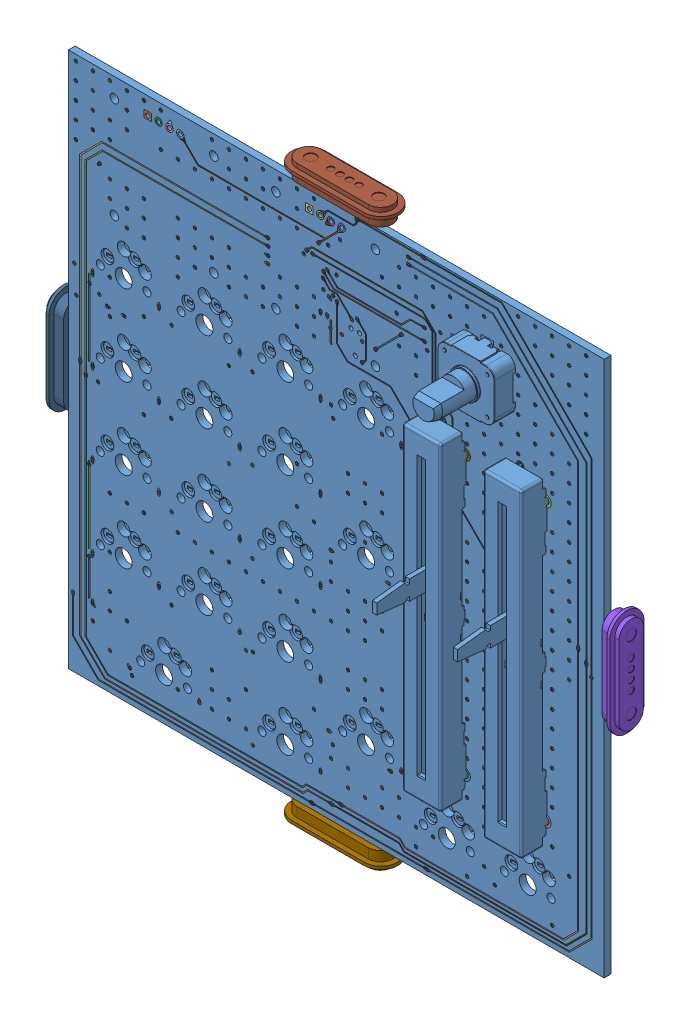
SolidWorks assembly Modulu1, configuration Default. Lengths in mm. (continued)
Components (placement in the parent): (continued)
- Numpad test 2.step-1: Numpad test 2.step [Default] at origin size (134.6 135 22.98) (continued)
  - Numpad test 21752.step-1: Numpad test 21752.step [Default] at origin size (1.31 0.29 0)
  - Numpad test 21753.step-1: Numpad test 21753.step [Default] at origin size (1.31 0.29 0)
  - Numpad test 21754.step-1: Numpad test 21754.step [Default] at origin size (0.82 0.18 0.01)
  - Numpad test 21755.step-1: Numpad test 21755.step [Default] at origin size (0.82 0.18 0.01)
  - Numpad test 21756.step-1: Numpad test 21756.step [Default] at origin size (1.76 0.36 0.01)
  - Numpad test 21757.step-1: Numpad test 21757.step [Default] at origin size (1.54 0.36 0.01)
  - Numpad test 21758.step-1: Numpad test 21758.step [Default] at origin size (0.38 0.64 0.01)
  - Numpad test 21759.step-1: Numpad test 21759.step [Default] at origin size (0.43 0.71 0.01)
  - Numpad test 21760.step-1: Numpad test 21760.step [Default] at origin size (2.14 1.77 0.01)
  - Numpad test 21761.step-1: Numpad test 21761.step [Default] at origin size (0.34 1.47 0.01)
  - Numpad test 21762.step-1: Numpad test 21762.step [Default] at origin size (0.34 1.47 0.01)
  - Numpad test 21763.step-1: Numpad test 21763.step [Default] at origin size (0.34 0.89 0.01)
  - Numpad test 21764.step-1: Numpad test 21764.step [Default] at origin size (0.34 0.89 0.01)
  - Numpad test 21765.step-1: Numpad test 21765.step [Default] at origin size (2.39 1.29 0.01)
  - Numpad test 21766.step-1: Numpad test 21766.step [Default] at origin size (2.33 1.32 0.01)
  - Numpad test 21767.step-1: Numpad test 21767.step [Default] at origin size (2.33 1.32 0.01)
  - Numpad test 21768.step-1: Numpad test 21768.step [Default] at origin size (2.33 1.32 0.01)
  - Numpad test 21769.step-1: Numpad test 21769.step [Default] at origin size (2.32 1.29 0.01)
  - Numpad test 21770.step-1: Numpad test 21770.step [Default] at origin size (2.3 1.29 0.01)
  - Numpad test 21771.step-1: Numpad test 21771.step [Default] at origin size (1.38 0.36 0.01)
  - Numpad test 21772.step-1: Numpad test 21772.step [Default] at origin size (0.36 0.71 0.01)
  - Numpad test 21773.step-1: Numpad test 21773.step [Default] at origin size (1.65 0.8 0.01)
  - Numpad test 21774.step-1: Numpad test 21774.step [Default] at origin size (2.15 1.25 0.02)
  - Numpad test 21775.step-1: Numpad test 21775.step [Default] at origin size (2.15 1.25 0.02)
  - Numpad test 21776.step-1: Numpad test 21776.step [Default] at origin size (2.15 1.25 0.02)
  - Numpad test 21777.step-1: Numpad test 21777.step [Default] at origin size (2.15 1.25 0.02)
  - Numpad test 21778.step-1: Numpad test 21778.step [Default] at origin size (2.15 1.25 0.02)
  - Numpad test 21779.step-1: Numpad test 21779.step [Default] at origin size (2.15 1.25 0.02)
  - Numpad test 21780.step-1: Numpad test 21780.step [Default] at origin size (2.15 1.25 0.02)
  - Numpad test 21781.step-1: Numpad test 21781.step [Default] at origin size (1.32 2.07 0.01)
  - Numpad test 21782.step-1: Numpad test 21782.step [Default] at origin size (1.19 0.27 0.01)
  - Numpad test 21783.step-1: Numpad test 21783.step [Default] at origin size (0.37 0.42 0.01)
  - Numpad test 21784.step-1: Numpad test 21784.step [Default] at origin size (1.26 0.4 0.01)
  - Numpad test 21785.step-1: Numpad test 21785.step [Default] at origin size (0.39 0.32 0.01)
  - Numpad test 21786.step-1: Numpad test 21786.step [Default] at origin size (0.09 0.09 0.01)
  - Numpad test 21787.step-1: Numpad test 21787.step [Default] at origin size (0.72 1.4 0)
  - Numpad test 21788.step-1: Numpad test 21788.step [Default] at origin size (0.72 1.42 0)
  - Numpad test 21789.step-1: Numpad test 21789.step [Default] at origin size (0.72 1.56 0)
  - Numpad test 21790.step-1: Numpad test 21790.step [Default] at origin size (0.72 1.56 0)
  - Numpad test 21791.step-1: Numpad test 21791.step [Default] at origin size (0.72 1.56 0)
  - Numpad test 21792.step-1: Numpad test 21792.step [Default] at origin size (0.72 1.56 0)
  - Numpad test 21793.step-1: Numpad test 21793.step [Default] at origin size (1.1 0.34 0.01)
  - Numpad test 21794.step-1: Numpad test 21794.step [Default] at origin size (0.36 0.33 0.01)
  - Numpad test 21795.step-1: Numpad test 21795.step [Default] at origin size (1.34 0.34 0.01)
  - Numpad test 21796.step-1: Numpad test 21796.step [Default] at origin size (0.2 0.37 0.01)
  - Numpad test 21797.step-1: Numpad test 21797.step [Default] at origin size (1.61 1.52 0.01)
  - Numpad test 21798.step-1: Numpad test 21798.step [Default] at origin size (1.38 1.39 0.01)
  - Numpad test 21799.step-1: Numpad test 21799.step [Default] at origin size (1.39 1.38 0.01)
  - Numpad test 21800.step-1: Numpad test 21800.step [Default] at origin size (1.28 0.37 0.01)
  - Numpad test 21801.step-1: Numpad test 21801.step [Default] at origin size (0.76 0.14 0.01)
  - Numpad test 21802.step-1: Numpad test 21802.step [Default] at origin size (0.32 0.77 0.01)
  - Numpad test 21803.step-1: Numpad test 21803.step [Default] at origin size (0.32 0.56 0.01)
  - Numpad test 21804.step-1: Numpad test 21804.step [Default] at origin size (1.45 1.59 0.01)
  - Numpad test 21805.step-1: Numpad test 21805.step [Default] at origin size (1.86 0.83 0.01)
  - Numpad test 21806.step-1: Numpad test 21806.step [Default] at origin size (0.61 1.43 0)
  - Numpad test 21807.step-1: Numpad test 21807.step [Default] at origin size (0.55 1.09 0)
  - Numpad test 21808.step-1: Numpad test 21808.step [Default] at origin size (0.8 1.02 0)
  - Numpad test 21809.step-1: Numpad test 21809.step [Default] at origin size (1.23 1.11 0)
  - Numpad test 21810.step-1: Numpad test 21810.step [Default] at origin size (1.69 0.83 0.01)
  - Numpad test 21811.step-1: Numpad test 21811.step [Default] at origin size (1.4 0.29 0.01)
  - Numpad test 21812.step-1: Numpad test 21812.step [Default] at origin size (1.4 0.29 0.01)
  - Numpad test 21813.step-1: Numpad test 21813.step [Default] at origin size (0.29 1.4 0.01)
  - Numpad test 21814.step-1: Numpad test 21814.step [Default] at origin size (0.29 1.4 0.01)
  - Numpad test 21815.step-1: Numpad test 21815.step [Default] at origin size (0.29 1.4 0.01)
  - Numpad test 21816.step-1: Numpad test 21816.step [Default] at origin size (0.29 1.4 0.01)
  - Numpad test 21817.step-1: Numpad test 21817.step [Default] at origin size (1.4 0.29 0.01)
  - Numpad test 21818.step-1: Numpad test 21818.step [Default] at origin size (1.4 0.29 0.01)
  - Numpad test 21819.step-1: Numpad test 21819.step [Default] at origin size (1.3 1.35 0.01)
  - Numpad test 21820.step-1: Numpad test 21820.step [Default] at origin size (1.51 1.08 0.01)
  - Numpad test 21821.step-1: Numpad test 21821.step [Default] at origin size (0.93 1.59 0.01)
  - Numpad test 21822.step-1: Numpad test 21822.step [Default] at origin size (0.78 0.71 0.01)
  - Numpad test 21823.step-1: Numpad test 21823.step [Default] at origin size (0.31 0.76 0.01)
  - Numpad test 21824.step-1: Numpad test 21824.step [Default] at origin size (0.83 0.29 0.01)
  - Numpad test 21825.step-1: Numpad test 21825.step [Default] at origin size (0.93 1.51 0.01)
  - Numpad test 21826.step-1: Numpad test 21826.step [Default] at origin size (0.66 0.37 0.01)
  - Numpad test 21827.step-1: Numpad test 21827.step [Default] at origin size (0.61 0.84 0.01)
  - Numpad test 21828.step-1: Numpad test 21828.step [Default] at origin size (0.83 0.72 0.01)
  - Numpad test 21829.step-1: Numpad test 21829.step [Default] at origin size (1.36 0.32 0)
  - Numpad test 21830.step-1: Numpad test 21830.step [Default] at origin size (1.36 0.32 0)
  - Numpad test 21831.step-1: Numpad test 21831.step [Default] at origin size (0.79 1.51 0.01)
  - Numpad test 21832.step-1: Numpad test 21832.step [Default] at origin size (0.93 1.41 0.01)
  - Numpad test 21833.step-1: Numpad test 21833.step [Default] at origin size (1.4 0.88 0.01)
  - Numpad test 21834.step-1: Numpad test 21834.step [Default] at origin size (1.17 0.32 0.01)
  - Numpad test 21835.step-1: Numpad test 21835.step [Default] at origin size (1.17 0.32 0.01)
  - Numpad test 21836.step-1: Numpad test 21836.step [Default] at origin size (1.4 0.88 0.01)
  - Numpad test 21837.step-1: Numpad test 21837.step [Default] at origin size (1.4 0.88 0.01)
  - Numpad test 21838.step-1: Numpad test 21838.step [Default] at origin size (1.4 0.88 0.01)
  - Numpad test 21839.step-1: Numpad test 21839.step [Default] at origin size (1.4 0.88 0.01)
  - Numpad test 21840.step-1: Numpad test 21840.step [Default] at origin size (1.4 0.88 0.01)
  - Numpad test 21841.step-1: Numpad test 21841.step [Default] at origin size (1.4 0.88 0.01)
  - Numpad test 21842.step-1: Numpad test 21842.step [Default] at origin size (1.17 0.32 0.01)
  - Numpad test 21843.step-1: Numpad test 21843.step [Default] at origin size (1.17 0.32 0.01)
  - Numpad test 21844.step-1: Numpad test 21844.step [Default] at origin size (1.4 0.88 0.01)
  - Numpad test 21845.step-1: Numpad test 21845.step [Default] at origin size (1.4 0.88 0.01)
  - Numpad test 21846.step-1: Numpad test 21846.step [Default] at origin size (1.4 0.88 0.01)
  - Numpad test 21847.step-1: Numpad test 21847.step [Default] at origin size (1.4 0.88 0.01)
  - Numpad test 21848.step-1: Numpad test 21848.step [Default] at origin size (1.4 0.88 0.01)
  - Numpad test 21849.step-1: Numpad test 21849.step [Default] at origin size (1.4 0.88 0.01)
  - Numpad test 21850.step-1: Numpad test 21850.step [Default] at origin size (1.4 0.88 0.01)
  - Numpad test 21851.step-1: Numpad test 21851.step [Default] at origin size (1.4 0.88 0.01)
  - Numpad test 21852.step-1: Numpad test 21852.step [Default] at origin size (1.4 0.88 0.01)
  - Numpad test 21853.step-1: Numpad test 21853.step [Default] at origin size (1.4 0.88 0.01)
  - Numpad test 21854.step-1: Numpad test 21854.step [Default] at origin size (1.4 0.88 0.01)
  - Numpad test 21855.step-1: Numpad test 21855.step [Default] at origin size (1.4 0.88 0.01)
  - Numpad test 21856.step-1: Numpad test 21856.step [Default] at origin size (1.4 0.88 0.01)
  - Numpad test 21857.step-1: Numpad test 21857.step [Default] at origin size (1.17 0.32 0.01)
  - Numpad test 21858.step-1: Numpad test 21858.step [Default] at origin size (1.17 0.32 0.01)
  - Numpad test 21859.step-1: Numpad test 21859.step [Default] at origin size (1.4 0.88 0.01)
  - Numpad test 21860.step-1: Numpad test 21860.step [Default] at origin size (1.17 0.32 0.01)
  - Numpad test 21861.step-1: Numpad test 21861.step [Default] at origin size (1.17 0.32 0.01)
  - Numpad test 21862.step-1: Numpad test 21862.step [Default] at origin size (1.4 0.88 0.01)
  - Numpad test 21863.step-1: Numpad test 21863.step [Default] at origin size (1.4 0.88 0.01)
  - Numpad test 21864.step-1: Numpad test 21864.step [Default] at origin size (1.4 0.88 0.01)
  - Numpad test 21865.step-1: Numpad test 21865.step [Default] at origin size (1.4 0.88 0.01)
  - Numpad test 21866.step-1: Numpad test 21866.step [Default] at origin size (1.4 0.88 0.01)
  - Numpad test 21867.step-1: Numpad test 21867.step [Default] at origin size (1.17 0.32 0.01)
  - Numpad test 21868.step-1: Numpad test 21868.step [Default] at origin size (1.17 0.32 0.01)
  - Numpad test 21869.step-1: Numpad test 21869.step [Default] at origin size (1.4 0.88 0.01)
  - Numpad test 21870.step-1: Numpad test 21870.step [Default] at origin size (1.4 0.88 0.01)
  - Numpad test 21871.step-1: Numpad test 21871.step [Default] at origin size (1.4 0.88 0.01)
  - Numpad test 21872.step-1: Numpad test 21872.step [Default] at origin size (1.4 0.88 0.01)
  - Numpad test 21873.step-1: Numpad test 21873.step [Default] at origin size (0.93 1.29 0.01)
  - Numpad test 21874.step-1: Numpad test 21874.step [Default] at origin size (0.93 1.29 0.01)
  - Numpad test 21875.step-1: Numpad test 21875.step [Default] at origin size (0.93 1.29 0.01)
  - Numpad test 21876.step-1: Numpad test 21876.step [Default] at origin size (0.93 1.29 0.01)
  - Numpad test 21877.step-1: Numpad test 21877.step [Default] at origin size (0.93 1.29 0.01)
  - Numpad test 21878.step-1: Numpad test 21878.step [Default] at origin size (0.93 1.29 0.01)
  - Numpad test 21879.step-1: Numpad test 21879.step [Default] at origin size (0.34 1.2 0)
  - Numpad test 21880.step-1: Numpad test 21880.step [Default] at origin size (0.34 1.2 0)
  - Numpad test 21881.step-1: Numpad test 21881.step [Default] at origin size (0.93 1.29 0.01)
  - Numpad test 21882.step-1: Numpad test 21882.step [Default] at origin size (0.93 1.21 0.01)
  - Numpad test 21883.step-1: Numpad test 21883.step [Default] at origin size (0.93 1.21 0.01)
  - Numpad test 21884.step-1: Numpad test 21884.step [Default] at origin size (0.93 1.21 0.01)
  - Numpad test 21885.step-1: Numpad test 21885.step [Default] at origin size (0.93 1.21 0.01)
  - Numpad test 21886.step-1: Numpad test 21886.step [Default] at origin size (0.93 1.19 0.01)
  - Numpad test 21887.step-1: Numpad test 21887.step [Default] at origin size (0.34 1.1 0)
  - Numpad test 21888.step-1: Numpad test 21888.step [Default] at origin size (0.34 1.1 0)
  - Numpad test 21889.step-1: Numpad test 21889.step [Default] at origin size (1.17 0.84 0.02)
  - Numpad test 21890.step-1: Numpad test 21890.step [Default] at origin size (0.72 0.18 0.01)
  - Numpad test 21891.step-1: Numpad test 21891.step [Default] at origin size (0.88 0.24 0.01)
  - Numpad test 21892.step-1: Numpad test 21892.step [Default] at origin size (1.18 0.59 0.01)
  - Numpad test 21893.step-1: Numpad test 21893.step [Default] at origin size (1.18 0.59 0.01)
  - Numpad test 21894.step-1: Numpad test 21894.step [Default] at origin size (1.18 0.59 0.01)
  - Numpad test 21895.step-1: Numpad test 21895.step [Default] at origin size (1.18 0.59 0.01)
  - Numpad test 21896.step-1: Numpad test 21896.step [Default] at origin size (1.18 0.59 0.01)
  - Numpad test 21897.step-1: Numpad test 21897.step [Default] at origin size (1.18 0.59 0.01)
  - Numpad test 21898.step-1: Numpad test 21898.step [Default] at origin size (0.88 0.24 0.01)
  - Numpad test 21899.step-1: Numpad test 21899.step [Default] at origin size (0.72 0.18 0.01)
  - Numpad test 21900.step-1: Numpad test 21900.step [Default] at origin size (0.61 1.11 0.01)
  - Numpad test 21901.step-1: Numpad test 21901.step [Default] at origin size (0.18 0.82 0.01)
  - Numpad test 21902.step-1: Numpad test 21902.step [Default] at origin size (0.18 0.82 0.01)
  - Numpad test 21903.step-1: Numpad test 21903.step [Default] at origin size (1.11 0.61 0.01)
  - Numpad test 21904.step-1: Numpad test 21904.step [Default] at origin size (0.18 0.82 0.01)
  - Numpad test 21905.step-1: Numpad test 21905.step [Default] at origin size (0.18 0.82 0.01)
  - Numpad test 21906.step-1: Numpad test 21906.step [Default] at origin size (0.18 0.82 0.01)
  - Numpad test 21907.step-1: Numpad test 21907.step [Default] at origin size (0.18 0.82 0.01)
  - Numpad test 21908.step-1: Numpad test 21908.step [Default] at origin size (1.11 0.61 0.01)
  - Numpad test 21909.step-1: Numpad test 21909.step [Default] at origin size (0.61 1.11 0.01)
  - Numpad test 21910.step-1: Numpad test 21910.step [Default] at origin size (0.18 0.82 0.01)
  - Numpad test 21911.step-1: Numpad test 21911.step [Default] at origin size (0.18 0.82 0.01)
  - Numpad test 21912.step-1: Numpad test 21912.step [Default] at origin size (1.11 0.61 0.01)
  - Numpad test 21913.step-1: Numpad test 21913.step [Default] at origin size (1.11 0.61 0.01)
  - Numpad test 21914.step-1: Numpad test 21914.step [Default] at origin size (1.11 0.61 0.01)
  - Numpad test 21915.step-1: Numpad test 21915.step [Default] at origin size (0.11 0.12 0.01)
  - Numpad test 21916.step-1: Numpad test 21916.step [Default] at origin size (0.11 0.56 0.01)
  - Numpad test 21917.step-1: Numpad test 21917.step [Default] at origin size (0.18 0.68 0.01)
  - Numpad test 21918.step-1: Numpad test 21918.step [Default] at origin size (0.63 0.34 0.01)
  - Numpad test 21919.step-1: Numpad test 21919.step [Default] at origin size (0.79 0.39 0.01)
  - Numpad test 21920.step-1: Numpad test 21920.step [Default] at origin size (0.63 0.34 0.01)
  - Numpad test 21921.step-1: Numpad test 21921.step [Default] at origin size (0.79 0.39 0.01)
  - Numpad test 21922.step-1: Numpad test 21922.step [Default] at origin size (0.91 0.84 0.01)
  - Numpad test 21923.step-1: Numpad test 21923.step [Default] at origin size (0.32 0.77 0.01)
  - Numpad test 21924.step-1: Numpad test 21924.step [Default] at origin size (0.32 0.77 0.01)
  - Numpad test 21925.step-1: Numpad test 21925.step [Default] at origin size (0.63 0.69 0.01)
  - Numpad test 21926.step-1: Numpad test 21926.step [Default] at origin size (0.57 0.5 0.01)
  - Numpad test 21927.step-1: Numpad test 21927.step [Default] at origin size (0.86 0.86 0.01)
  - Numpad test 21928.step-1: Numpad test 21928.step [Default] at origin size (0.86 0.86 0.01)
  - Numpad test 21929.step-1: Numpad test 21929.step [Default] at origin size (0.5 0.67 0)
  - Numpad test 21930.step-1: Numpad test 21930.step [Default] at origin size (0.67 0.5 0)
  - Numpad test 21931.step-1: Numpad test 21931.step [Default] at origin size (0.67 0.5 0)
  - Numpad test 21932.step-1: Numpad test 21932.step [Default] at origin size (0.5 0.67 0)
  - Numpad test 21933.step-1: Numpad test 21933.step [Default] at origin size (0.5 0.67 0)
  - Numpad test 21934.step-1: Numpad test 21934.step [Default] at origin size (0.67 0.5 0)
  - Numpad test 21935.step-1: Numpad test 21935.step [Default] at origin size (0.5 0.67 0)
  - Numpad test 21936.step-1: Numpad test 21936.step [Default] at origin size (0.67 0.5 0)
  - Numpad test 21937.step-1: Numpad test 21937.step [Default] at origin size (0.5 0.67 0)
  - Numpad test 21938.step-1: Numpad test 21938.step [Default] at origin size (0.67 0.5 0)
  - Numpad test 21939.step-1: Numpad test 21939.step [Default] at origin size (0.67 0.5 0)
  - Numpad test 21940.step-1: Numpad test 21940.step [Default] at origin size (0.5 0.67 0)
  - Numpad test 21941.step-1: Numpad test 21941.step [Default] at origin size (0.86 0.86 0.01)
  - Numpad test 21942.step-1: Numpad test 21942.step [Default] at origin size (0.86 0.86 0.01)
  - Numpad test 21943.step-1: Numpad test 21943.step [Default] at origin size (0.53 0.65 0.01)
  - Numpad test 21944.step-1: Numpad test 21944.step [Default] at origin size (0.69 0.47 0)
  - Numpad test 21945.step-1: Numpad test 21945.step [Default] at origin size (0.31 0.76 0.01)
  - Numpad test 21946.step-1: Numpad test 21946.step [Default] at origin size (0.31 0.76 0.01)
  - Numpad test 21947.step-1: Numpad test 21947.step [Default] at origin size (0.76 0.31 0.01)
  - Numpad test 21948.step-1: Numpad test 21948.step [Default] at origin size (0.76 0.31 0.01)
  - Numpad test 21949.step-1: Numpad test 21949.step [Default] at origin size (0.86 0.85 0.01)
  - Numpad test 21950.step-1: Numpad test 21950.step [Default] at origin size (0.75 0.31 0.01)
  - Numpad test 21951.step-1: Numpad test 21951.step [Default] at origin size (0.75 0.31 0.01)
  - Numpad test 21952.step-1: Numpad test 21952.step [Default] at origin size (0.85 0.86 0.01)
  - Numpad test 21953.step-1: Numpad test 21953.step [Default] at origin size (0.51 0.69 0.01)
  - Numpad test 21954.step-1: Numpad test 21954.step [Default] at origin size (0.03 0.21 0.01)
  - Numpad test 21955.step-1: Numpad test 21955.step [Default] at origin size (0.37 0.44 0.01)
  - Numpad test 21956.step-1: Numpad test 21956.step [Default] at origin size (0.57 0.67 0.01)
  - Numpad test 21957.step-1: Numpad test 21957.step [Default] at origin size (0.63 0.57 0.01)
  - Numpad test 21958.step-1: Numpad test 21958.step [Default] at origin size (0.8 0.27 0.01)
  - Numpad test 21959.step-1: Numpad test 21959.step [Default] at origin size (0.8 0.27 0.01)
  - Numpad test 21960.step-1: Numpad test 21960.step [Default] at origin size (0.8 0.27 0.01)
  - Numpad test 21961.step-1: Numpad test 21961.step [Default] at origin size (0.8 0.27 0.01)
  - Numpad test 21962.step-1: Numpad test 21962.step [Default] at origin size (0.85 0.78 0.01)
  - Numpad test 21963.step-1: Numpad test 21963.step [Default] at origin size (0.8 0.27 0.01)
  - Numpad test 21964.step-1: Numpad test 21964.step [Default] at origin size (0.8 0.27 0.01)
  - Numpad test 21965.step-1: Numpad test 21965.step [Default] at origin size (0.83 0.79 0.01)
  - Numpad test 21966.step-1: Numpad test 21966.step [Default] at origin size (0.79 0.81 0.01)
  - Numpad test 21967.step-1: Numpad test 21967.step [Default] at origin size (0.79 0.81 0.01)
  - Numpad test 21968.step-1: Numpad test 21968.step [Default] at origin size (0.77 0.29 0)
  - Numpad test 21969.step-1: Numpad test 21969.step [Default] at origin size (0.77 0.29 0)
  - Numpad test 21970.step-1: Numpad test 21970.step [Default] at origin size (0.78 0.79 0.01)
  - Numpad test 21971.step-1: Numpad test 21971.step [Default] at origin size (0.78 0.79 0.01)
  - Numpad test 21972.step-1: Numpad test 21972.step [Default] at origin size (0.78 0.79 0.01)
  - Numpad test 21973.step-1: Numpad test 21973.step [Default] at origin size (0.77 0.29 0)
  - Numpad test 21974.step-1: Numpad test 21974.step [Default] at origin size (0.77 0.29 0)
  - Numpad test 21975.step-1: Numpad test 21975.step [Default] at origin size (0.78 0.79 0.01)
  - Numpad test 21976.step-1: Numpad test 21976.step [Default] at origin size (0.78 0.79 0.01)
  - Numpad test 21977.step-1: Numpad test 21977.step [Default] at origin size (0.78 0.79 0.01)
  - Numpad test 21978.step-1: Numpad test 21978.step [Default] at origin size (0.78 0.79 0.01)
  - Numpad test 21979.step-1: Numpad test 21979.step [Default] at origin size (0.78 0.79 0.01)
  - Numpad test 21980.step-1: Numpad test 21980.step [Default] at origin size (0.78 0.79 0.01)
  - Numpad test 21981.step-1: Numpad test 21981.step [Default] at origin size (0.78 0.79 0.01)
  - Numpad test 21982.step-1: Numpad test 21982.step [Default] at origin size (0.77 0.29 0)
  - Numpad test 21983.step-1: Numpad test 21983.step [Default] at origin size (0.77 0.29 0)
  - Numpad test 21984.step-1: Numpad test 21984.step [Default] at origin size (0.77 0.29 0)
  - Numpad test 21985.step-1: Numpad test 21985.step [Default] at origin size (0.77 0.29 0)
  - Numpad test 21986.step-1: Numpad test 21986.step [Default] at origin size (0.78 0.79 0.01)
  - Numpad test 21987.step-1: Numpad test 21987.step [Default] at origin size (0.73 0.29 0)
  - Numpad test 21988.step-1: Numpad test 21988.step [Default] at origin size (0.77 0.29 0)
  - Numpad test 21989.step-1: Numpad test 21989.step [Default] at origin size (0.77 0.29 0)
  - Numpad test 21990.step-1: Numpad test 21990.step [Default] at origin size (0.77 0.29 0)
  - Numpad test 21991.step-1: Numpad test 21991.step [Default] at origin size (0.78 0.79 0.01)
  - Numpad test 21992.step-1: Numpad test 21992.step [Default] at origin size (0.78 0.79 0.01)
  - Numpad test 21993.step-1: Numpad test 21993.step [Default] at origin size (0.77 0.29 0)
  - Numpad test 21994.step-1: Numpad test 21994.step [Default] at origin size (0.77 0.29 0)
  - Numpad test 21995.step-1: Numpad test 21995.step [Default] at origin size (0.78 0.79 0.01)
  - Numpad test 21996.step-1: Numpad test 21996.step [Default] at origin size (0.78 0.79 0.01)
  - Numpad test 21997.step-1: Numpad test 21997.step [Default] at origin size (0.28 0.77 0)
  - Numpad test 21998.step-1: Numpad test 21998.step [Default] at origin size (0.28 0.77 0)
  - Numpad test 21999.step-1: Numpad test 21999.step [Default] at origin size (0.28 0.77 0)
  - Numpad test 22000.step-1: Numpad test 22000.step [Default] at origin size (0.28 0.77 0)
  - Numpad test 22001.step-1: Numpad test 22001.step [Default] at origin size (0.28 0.77 0)
  - Numpad test 22002.step-1: Numpad test 22002.step [Default] at origin size (0.28 0.77 0)
  - Numpad test 22003.step-1: Numpad test 22003.step [Default] at origin size (0.28 0.77 0)
  - Numpad test 22004.step-1: Numpad test 22004.step [Default] at origin size (0.28 0.77 0)
  - Numpad test 22005.step-1: Numpad test 22005.step [Default] at origin size (0.28 0.77 0)
  - Numpad test 22006.step-1: Numpad test 22006.step [Default] at origin size (0.28 0.77 0)
  - Numpad test 22007.step-1: Numpad test 22007.step [Default] at origin size (0.28 0.77 0)
  - Numpad test 22008.step-1: Numpad test 22008.step [Default] at origin size (0.28 0.77 0)
  - Numpad test 22009.step-1: Numpad test 22009.step [Default] at origin size (0.67 0.53 0)
  - Numpad test 22010.step-1: Numpad test 22010.step [Default] at origin size (0.63 0.32 0)
  - Numpad test 22011.step-1: Numpad test 22011.step [Default] at origin size (0.54 0.48 0.01)
  - Numpad test 22012.step-1: Numpad test 22012.step [Default] at origin size (0.43 0.33 0.01)
  - Numpad test 22013.step-1: Numpad test 22013.step [Default] at origin size (0.73 0.69 0.01)
  - Numpad test 22014.step-1: Numpad test 22014.step [Default] at origin size (0.45 0.49 0)
  - Numpad test 22015.step-1: Numpad test 22015.step [Default] at origin size (0.03 0.16 0.01)
  - Numpad test 22016.step-1: Numpad test 22016.step [Default] at origin size (0.29 0.34 0)
  - Numpad test 22017.step-1: Numpad test 22017.step [Default] at origin size (0.4 0.12 0.01)
  - Numpad test 22018.step-1: Numpad test 22018.step [Default] at origin size (0.5 0.27 0.01)
  - Numpad test 22019.step-1: Numpad test 22019.step [Default] at origin size (0.23 0.5 0.01)
  - Numpad test 22020.step-1: Numpad test 22020.step [Default] at origin size (0.17 0.34 0.01)
  - Numpad test 22021.step-1: Numpad test 22021.step [Default] at origin size (0.26 0.46 0.01)
  - Numpad test 22022.step-1: Numpad test 22022.step [Default] at origin size (0.22 0.33 0.01)
  - Numpad test 22023.step-1: Numpad test 22023.step [Default] at origin size (0.44 0.62 0.01)
  - Numpad test 22024.step-1: Numpad test 22024.step [Default] at origin size (5 25 8)
  - Numpad test 22025.step-1: Numpad test 22025.step [Default] at origin size (25 5 8)
  - Numpad test 22026.step-1: Numpad test 22026.step [Default] at origin size (5 25 8)
  - Numpad test 22027.step-1: Numpad test 22027.step [Default] at origin size (25 5 8)
